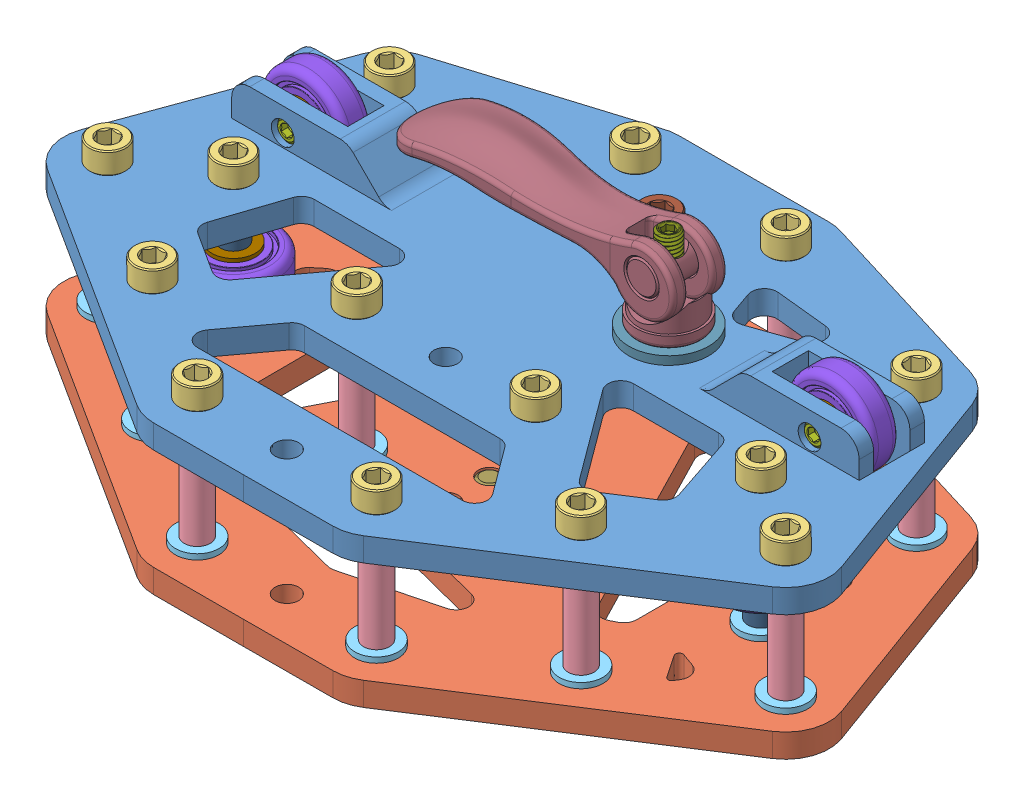
SolidWorks assembly Z-Carriage_Right, configuration Default. Lengths in mm.
Overall size (211.06 78.88 141.66).
122 component instances, 16 part files, 42 mates.
Components (placement in the parent):
- Z_Carriage_Roller_Plate_Top_B-1: Z_Carriage_Roller_Plate_Top_B [Default] at (-57.0039 2.4125 0.8021) size (210.67 16.5 141.06)
- Z_Carriage_Roller_Plate_Bottom_B-1: Z_Carriage_Roller_Plate_Bottom_B [Default] at (-56.8663 -25.5875 0.8019) x (-0.999996 0 0.002837) z (0.002837 0 0.999996) size (210.67 6.5 141.06)
- Z-Carriage_Bolt_Standoff_Assembly-1: Z-Carriage_Bolt_Standoff_Assembly [Default] at (-155.6945 -13.6491 33.5414) x (0.864384 0 -0.502833) z (0 -1 0) size (13.84 13.84 47.54)
  - 40mm_M6_Bolt-1: 40mm_M6_Bolt [96144A140] at (2.8443 6.0053 17.4384) size (10 10 46.54)
  - Z-Carriage_Standoff-1: Z-Carriage_Standoff [Default] at (2.8443 6.0053 10.4384) x (0.794662 -0.607053 0) z (0.607053 0.794662 0) size (7.14 25 7.14)
  - M6_1.5mmT_Washer-2: M6_1.5mmT_Washer [Default] at (2.8443 6.0053 -14.5616) x (1 0 0) z (0 1 0) size (12 1.5 12)
  - M6_1.5mmT_Washer-3: M6_1.5mmT_Washer [Default] at (2.8443 6.0053 11.9384) x (0.985875 0.167484 0) z (-0.167484 0.985875 0) size (12 1.5 12)
  - Nut_M6-1: Nut_M6 [91415A040] at (2.8443 6.0053 15.9384) size (10 11.55 5.56)
- Z-Carriage_Bolt_Standoff_Assembly-2: Z-Carriage_Bolt_Standoff_Assembly [Default] at (-121.3383 -13.7531 55.5414) x (0.864384 0 -0.502833) z (0 -1 0) size (13.84 13.84 47.54)
  - 40mm_M6_Bolt-1: 40mm_M6_Bolt [96144A140] at (2.8443 6.0053 17.4384) size (10 10 46.54)
  - Z-Carriage_Standoff-1: Z-Carriage_Standoff [Default] at (2.8443 6.0053 10.4384) x (0.794662 -0.607053 0) z (0.607053 0.794662 0) size (7.14 25 7.14)
  - M6_1.5mmT_Washer-2: M6_1.5mmT_Washer [Default] at (2.8443 6.0053 -14.5616) x (1 0 0) z (0 1 0) size (12 1.5 12)
  - M6_1.5mmT_Washer-3: M6_1.5mmT_Washer [Default] at (2.8443 6.0053 11.9384) x (0.985875 0.167484 0) z (-0.167484 0.985875 0) size (12 1.5 12)
  - Nut_M6-1: Nut_M6 [91415A040] at (2.8443 6.0053 15.9384) size (10 11.55 5.56)
- Z-Carriage_Bolt_Standoff_Assembly-3: Z-Carriage_Bolt_Standoff_Assembly [Default] at (-88.0491 -13.6491 80.1556) x (0.577555 0 -0.816352) z (0 -1 0) size (13.84 13.84 47.54)
  - 40mm_M6_Bolt-1: 40mm_M6_Bolt [96144A140] at (2.8443 6.0053 17.4384) size (10 10 46.54)
  - Z-Carriage_Standoff-1: Z-Carriage_Standoff [Default] at (2.8443 6.0053 10.4384) x (0.794662 -0.607053 0) z (0.607053 0.794662 0) size (7.14 25 7.14)
  - M6_1.5mmT_Washer-2: M6_1.5mmT_Washer [Default] at (2.8443 6.0053 -14.5616) x (1 0 0) z (0 1 0) size (12 1.5 12)
  - M6_1.5mmT_Washer-3: M6_1.5mmT_Washer [Default] at (2.8443 6.0053 11.9384) x (0.985875 0.167484 0) z (-0.167484 0.985875 0) size (12 1.5 12)
  - Nut_M6-1: Nut_M6 [91415A040] at (2.8443 6.0053 15.9384) size (10 11.55 5.56)
- Z-Carriage_Bolt_Standoff_Assembly-4: Z-Carriage_Bolt_Standoff_Assembly [Default] at (-37.6163 -13.6491 77.4714) x (0.864384 0 -0.502833) z (0 -1 0) size (13.84 13.84 47.54)
  - 40mm_M6_Bolt-1: 40mm_M6_Bolt [96144A140] at (2.8443 6.0053 17.4384) size (10 10 46.54)
  - Z-Carriage_Standoff-1: Z-Carriage_Standoff [Default] at (2.8443 6.0053 10.4384) x (0.794662 -0.607053 0) z (0.607053 0.794662 0) size (7.14 25 7.14)
  - M6_1.5mmT_Washer-2: M6_1.5mmT_Washer [Default] at (2.8443 6.0053 -14.5616) x (1 0 0) z (0 1 0) size (12 1.5 12)
  - M6_1.5mmT_Washer-3: M6_1.5mmT_Washer [Default] at (2.8443 6.0053 11.9384) x (0.985875 0.167484 0) z (-0.167484 0.985875 0) size (12 1.5 12)
  - Nut_M6-1: Nut_M6 [91415A040] at (2.8443 6.0053 15.9384) size (10 11.55 5.56)
- Z-Carriage_Bolt_Standoff_Assembly-5: Z-Carriage_Bolt_Standoff_Assembly [Default] at (-3.3227 -13.6491 55.374) x (0.864384 0 -0.502833) z (0 -1 0) size (13.84 13.84 47.54)
  - 40mm_M6_Bolt-1: 40mm_M6_Bolt [96144A140] at (2.8443 6.0053 17.4384) size (10 10 46.54)
  - Z-Carriage_Standoff-1: Z-Carriage_Standoff [Default] at (2.8443 6.0053 10.4384) x (0.794662 -0.607053 0) z (0.607053 0.794662 0) size (7.14 25 7.14)
  - M6_1.5mmT_Washer-2: M6_1.5mmT_Washer [Default] at (2.8443 6.0053 -14.5616) x (1 0 0) z (0 1 0) size (12 1.5 12)
  - M6_1.5mmT_Washer-3: M6_1.5mmT_Washer [Default] at (2.8443 6.0053 11.9384) x (0.985875 0.167484 0) z (-0.167484 0.985875 0) size (12 1.5 12)
  - Nut_M6-1: Nut_M6 [91415A040] at (2.8443 6.0053 15.9384) size (10 11.55 5.56)
- Z-Carriage_Bolt_Standoff_Assembly-6: Z-Carriage_Bolt_Standoff_Assembly [Default] at (30.9709 -13.6491 33.2766) x (0.864384 0 -0.502833) z (0 -1 0) size (13.84 13.84 47.54)
  - 40mm_M6_Bolt-1: 40mm_M6_Bolt [96144A140] at (2.8443 6.0053 17.4384) size (10 10 46.54)
  - Z-Carriage_Standoff-1: Z-Carriage_Standoff [Default] at (2.8443 6.0053 10.4384) x (0.794662 -0.607053 0) z (0.607053 0.794662 0) size (7.14 25 7.14)
  - M6_1.5mmT_Washer-2: M6_1.5mmT_Washer [Default] at (2.8443 6.0053 -14.5616) x (1 0 0) z (0 1 0) size (12 1.5 12)
  - M6_1.5mmT_Washer-3: M6_1.5mmT_Washer [Default] at (2.8443 6.0053 11.9384) x (0.985875 0.167484 0) z (-0.167484 0.985875 0) size (12 1.5 12)
  - Nut_M6-1: Nut_M6 [91415A040] at (2.8443 6.0053 15.9384) size (10 11.55 5.56)
- Z-Carriage_Bolt_Standoff_Assembly-7: Z-Carriage_Bolt_Standoff_Assembly [Default] at (-30.9693 -13.6491 -39.7802) x (0.206565 0 0.978433) z (0 -1 0) size (13.84 13.84 47.54)
  - 40mm_M6_Bolt-1: 40mm_M6_Bolt [96144A140] at (2.8443 6.0053 17.4384) size (10 10 46.54)
  - Z-Carriage_Standoff-1: Z-Carriage_Standoff [Default] at (2.8443 6.0053 10.4384) x (0.794662 -0.607053 0) z (0.607053 0.794662 0) size (7.14 25 7.14)
  - M6_1.5mmT_Washer-2: M6_1.5mmT_Washer [Default] at (2.8443 6.0053 -14.5616) x (1 0 0) z (0 1 0) size (12 1.5 12)
  - M6_1.5mmT_Washer-3: M6_1.5mmT_Washer [Default] at (2.8443 6.0053 11.9384) x (0.985875 0.167484 0) z (-0.167484 0.985875 0) size (12 1.5 12)
  - Nut_M6-1: Nut_M6 [91415A040] at (2.8443 6.0053 15.9384) size (10 11.55 5.56)
- Z-Carriage_Bolt_Standoff_Assembly-8: Z-Carriage_Bolt_Standoff_Assembly [Default] at (-83.1945 -13.6491 -39.4586) x (0.864384 0 -0.502833) z (0 -1 0) size (13.84 13.84 47.54)
  - 40mm_M6_Bolt-1: 40mm_M6_Bolt [96144A140] at (2.8443 6.0053 17.4384) size (10 10 46.54)
  - Z-Carriage_Standoff-1: Z-Carriage_Standoff [Default] at (2.8443 6.0053 10.4384) x (0.794662 -0.607053 0) z (0.607053 0.794662 0) size (7.14 25 7.14)
  - M6_1.5mmT_Washer-2: M6_1.5mmT_Washer [Default] at (2.8443 6.0053 -14.5616) x (1 0 0) z (0 1 0) size (12 1.5 12)
  - M6_1.5mmT_Washer-3: M6_1.5mmT_Washer [Default] at (2.8443 6.0053 11.9384) x (0.985875 0.167484 0) z (-0.167484 0.985875 0) size (12 1.5 12)
  - Nut_M6-1: Nut_M6 [91415A040] at (2.8443 6.0053 15.9384) size (10 11.55 5.56)
- Z-Carriage_Bolt_Standoff_Assembly-9: Z-Carriage_Bolt_Standoff_Assembly [Default] at (-86.9821 -13.6491 33.5414) x (0.864384 0 -0.502833) z (0 -1 0) size (13.84 13.84 47.54)
  - 40mm_M6_Bolt-1: 40mm_M6_Bolt [96144A140] at (2.8443 6.0053 17.4384) size (10 10 46.54)
  - Z-Carriage_Standoff-1: Z-Carriage_Standoff [Default] at (2.8443 6.0053 10.4384) x (0.794662 -0.607053 0) z (0.607053 0.794662 0) size (7.14 25 7.14)
  - M6_1.5mmT_Washer-2: M6_1.5mmT_Washer [Default] at (2.8443 6.0053 -14.5616) x (1 0 0) z (0 1 0) size (12 1.5 12)
  - M6_1.5mmT_Washer-3: M6_1.5mmT_Washer [Default] at (2.8443 6.0053 11.9384) x (0.985875 0.167484 0) z (-0.167484 0.985875 0) size (12 1.5 12)
  - Nut_M6-1: Nut_M6 [91415A040] at (2.8443 6.0053 15.9384) size (10 11.55 5.56)
- Z-Carriage_Bolt_Standoff_Assembly-10: Z-Carriage_Bolt_Standoff_Assembly [Default] at (-37.7411 -13.6491 33.4715) x (0.864384 0 -0.502833) z (0 -1 0) size (13.84 13.84 47.54)
  - 40mm_M6_Bolt-1: 40mm_M6_Bolt [96144A140] at (2.8443 6.0053 17.4384) size (10 10 46.54)
  - Z-Carriage_Standoff-1: Z-Carriage_Standoff [Default] at (2.8443 6.0053 10.4384) x (0.794662 -0.607053 0) z (0.607053 0.794662 0) size (7.14 25 7.14)
  - M6_1.5mmT_Washer-2: M6_1.5mmT_Washer [Default] at (2.8443 6.0053 -14.5616) x (1 0 0) z (0 1 0) size (12 1.5 12)
  - M6_1.5mmT_Washer-3: M6_1.5mmT_Washer [Default] at (2.8443 6.0053 11.9384) x (0.985875 0.167484 0) z (-0.167484 0.985875 0) size (12 1.5 12)
  - Nut_M6-1: Nut_M6 [91415A040] at (2.8443 6.0053 15.9384) size (10 11.55 5.56)
- Z-Carriage_Bolt_Standoff_Assembly-11: Z-Carriage_Bolt_Standoff_Assembly [Default] at (-135.6486 -13.6491 -17.1687) x (0.051837 0 -0.998656) z (0 -1 0) size (13.84 13.84 47.54)
  - 40mm_M6_Bolt-1: 40mm_M6_Bolt [96144A140] at (2.8443 6.0053 17.4384) size (10 10 46.54)
  - Z-Carriage_Standoff-1: Z-Carriage_Standoff [Default] at (2.8443 6.0053 10.4384) x (0.794662 -0.607053 0) z (0.607053 0.794662 0) size (7.14 25 7.14)
  - M6_1.5mmT_Washer-2: M6_1.5mmT_Washer [Default] at (2.8443 6.0053 -14.5616) x (1 0 0) z (0 1 0) size (12 1.5 12)
  - M6_1.5mmT_Washer-3: M6_1.5mmT_Washer [Default] at (2.8443 6.0053 11.9384) x (0.985875 0.167484 0) z (-0.167484 0.985875 0) size (12 1.5 12)
  - Nut_M6-1: Nut_M6 [91415A040] at (2.8443 6.0053 15.9384) size (10 11.55 5.56)
- Z-Carriage_Bolt_Standoff_Assembly-12: Z-Carriage_Bolt_Standoff_Assembly [Default] at (18.6675 -13.6491 -25.7853) x (0.600743 0 0.799443) z (0 -1 0) size (13.84 13.84 47.54)
  - 40mm_M6_Bolt-1: 40mm_M6_Bolt [96144A140] at (2.8443 6.0053 17.4384) size (10 10 46.54)
  - Z-Carriage_Standoff-1: Z-Carriage_Standoff [Default] at (2.8443 6.0053 10.4384) x (0.794662 -0.607053 0) z (0.607053 0.794662 0) size (7.14 25 7.14)
  - M6_1.5mmT_Washer-2: M6_1.5mmT_Washer [Default] at (2.8443 6.0053 -14.5616) x (1 0 0) z (0 1 0) size (12 1.5 12)
  - M6_1.5mmT_Washer-3: M6_1.5mmT_Washer [Default] at (2.8443 6.0053 11.9384) x (0.985875 0.167484 0) z (-0.167484 0.985875 0) size (12 1.5 12)
  - Nut_M6-1: Nut_M6 [91415A040] at (2.8443 6.0053 15.9384) size (10 11.55 5.56)
- Top_Bearing_Assembly-1: Top_Bearing_Assembly [Default] at (10.689 4.0604 -12.7646) size (24 24 17)
  - M6_Top_Bearing_Setscrew-1: M6_Top_Bearing_Setscrew [91390A132] at (5.1177 8.3521 14.0605) size (6.22 6.16 17)
  - Roller_Bearing_Placeholder-1: Roller_Bearing_Placeholder [Default] at (5.1177 8.3521 9.5666) x (1 0 0) z (0 -1 0) size (24 8 24)
  - M6_1mmT_Washer-1: M6_1mmT_Washer [Default] at (5.1177 8.3521 17.5666) x (-0.598252 0.801308 0) z (0.801308 0.598252 0) size (12 1 12)
  - M6_1mmT_Washer-2: M6_1mmT_Washer [Default] at (5.1177 8.3521 8.5666) x (0.928702 -0.370827 0) z (-0.370827 -0.928702 0) size (12 1 12)
- Top_Bearing_Assembly-2: Top_Bearing_Assembly [Default] at (-134.5321 4.0604 -12.7646) size (24 24 17)
  - M6_Top_Bearing_Setscrew-1: M6_Top_Bearing_Setscrew [91390A132] at (5.1177 8.3521 14.0605) size (6.22 6.16 17)
  - Roller_Bearing_Placeholder-1: Roller_Bearing_Placeholder [Default] at (5.1177 8.3521 9.5666) x (1 0 0) z (0 -1 0) size (24 8 24)
  - M6_1mmT_Washer-1: M6_1mmT_Washer [Default] at (5.1177 8.3521 17.5666) x (-0.598252 0.801308 0) z (0.801308 0.598252 0) size (12 1 12)
  - M6_1mmT_Washer-2: M6_1mmT_Washer [Default] at (5.1177 8.3521 8.5666) x (0.928702 -0.370827 0) z (-0.370827 -0.928702 0) size (12 1 12)
- Side_Bearing_Assembly-1: Side_Bearing_Assembly [Default] at (-125.5625 18.7773 -11.5921) x (0.874247 0 -0.485481) z (0.485463 -0.008727 0.874214) size (24.63 47.63 24.7)
  - 40mm_M6_Bolt-1: 40mm_M6_Bolt [96144A140] at (-20.3862 -49.6134 29.0267) x (1 0 0) z (0 -0.999962 0.008727) size (10 10 46.54)
  - M6_1.5mmT_Washer-1: M6_1.5mmT_Washer [Default] at (-20.3862 -17.6146 28.7474) x (1 0 0) z (0 0.008727 0.999962) size (12 1.5 12)
  - Roller_Bearing_Placeholder-1: Roller_Bearing_Placeholder [Default] at (-20.3862 -34.114 28.8914) x (0.999646 -0.000232 -0.026596) z (0.026597 0.008723 0.999608) size (24 8 24)
  - Z-Carriage_Standoff_Bearing-1: Z-Carriage_Standoff_Bearing [Default] at (-20.3862 -25.1143 28.8129) x (1 0 0) z (0 0.008727 0.999962) size (7.14 7.5 7.14)
  - M6_1mmT_Washer-1: M6_1mmT_Washer [Default] at (-20.3862 -26.1143 28.8216) x (0.997316 -0.000639 -0.073218) z (0.07322 0.008703 0.997278) size (12 1 12)
  - M6_1mmT_Washer-3: M6_1mmT_Washer [Default] at (-20.3862 -35.114 28.9001) x (0.947667 0.002786 0.319249) z (-0.319261 0.00827 0.947631) size (12 1 12)
  - Z-Carriage_Standoff_Bearing-3: Z-Carriage_Standoff_Bearing [Default] at (-20.3862 -42.6137 28.9656) x (1 0 0) z (0 0.008727 0.999962) size (7.14 7.5 7.14)
  - M6_1.5mmT_Washer-3: M6_1.5mmT_Washer [Default] at (-20.3862 -44.1136 28.9787) x (1 0 0) z (0 0.008727 0.999962) size (12 1.5 12)
  - Nut_M6-1: Nut_M6 [91415A040] at (-20.3862 -48.1135 29.0136) x (0.999124 -0.000365 -0.041848) z (0 -0.999962 0.008727) size (10 11.55 5.56)
- Side_Bearing_Assembly-2: Side_Bearing_Assembly [Default] at (19.6386 18.7773 -11.798) x (0.874247 0 -0.485481) z (0.485463 -0.008727 0.874214) size (24.63 47.63 24.7)
  - 40mm_M6_Bolt-1: 40mm_M6_Bolt [96144A140] at (-20.3862 -49.6134 29.0267) x (1 0 0) z (0 -0.999962 0.008727) size (10 10 46.54)
  - M6_1.5mmT_Washer-1: M6_1.5mmT_Washer [Default] at (-20.3862 -17.6146 28.7474) x (1 0 0) z (0 0.008727 0.999962) size (12 1.5 12)
  - Roller_Bearing_Placeholder-1: Roller_Bearing_Placeholder [Default] at (-20.3862 -34.114 28.8914) x (0.999646 -0.000232 -0.026596) z (0.026597 0.008723 0.999608) size (24 8 24)
  - Z-Carriage_Standoff_Bearing-1: Z-Carriage_Standoff_Bearing [Default] at (-20.3862 -25.1143 28.8129) x (1 0 0) z (0 0.008727 0.999962) size (7.14 7.5 7.14)
  - M6_1mmT_Washer-1: M6_1mmT_Washer [Default] at (-20.3862 -26.1143 28.8216) x (0.997316 -0.000639 -0.073218) z (0.07322 0.008703 0.997278) size (12 1 12)
  - M6_1mmT_Washer-3: M6_1mmT_Washer [Default] at (-20.3862 -35.114 28.9001) x (0.947667 0.002786 0.319249) z (-0.319261 0.00827 0.947631) size (12 1 12)
  - Z-Carriage_Standoff_Bearing-3: Z-Carriage_Standoff_Bearing [Default] at (-20.3862 -42.6137 28.9656) x (1 0 0) z (0 0.008727 0.999962) size (7.14 7.5 7.14)
  - M6_1.5mmT_Washer-3: M6_1.5mmT_Washer [Default] at (-20.3862 -44.1136 28.9787) x (1 0 0) z (0 0.008727 0.999962) size (12 1.5 12)
  - Nut_M6-1: Nut_M6 [91415A040] at (-20.3862 -48.1135 29.0136) x (0.999124 -0.000365 -0.041848) z (0 -0.999962 0.008727) size (10 11.55 5.56)
- Idler_Bearing_Assembly-1: Idler_Bearing_Assembly [Default] at (-86.4176 18.7773 -2.3736) x (-0.930317 0 -0.366758) z (0.366744 -0.008727 -0.930281) size (24.63 56.64 24.7)
  - M6_1.5mmT_Washer-1: M6_1.5mmT_Washer [Default] at (-20.3135 -17.6139 28.8293) x (1 0 0) z (0 0.008727 0.999962) size (12 1.5 12)
  - Roller_Bearing_Placeholder-1: Roller_Bearing_Placeholder [Default] at (-20.3135 -34.1133 28.9733) x (0.999646 -0.000232 -0.026596) z (0.026597 0.008723 0.999608) size (24 8 24)
  - Z-Carriage_Standoff_Bearing-1: Z-Carriage_Standoff_Bearing [Default] at (-20.3135 -25.1136 28.8947) x (1 0 0) z (0 0.008727 0.999962) size (7.14 7.5 7.14)
  - M6_1mmT_Washer-1: M6_1mmT_Washer [Default] at (-20.3135 -26.1136 28.9035) x (0.997316 -0.000639 -0.073218) z (0.07322 0.008703 0.997278) size (12 1 12)
  - M6_1mmT_Washer-3: M6_1mmT_Washer [Default] at (-20.3135 -35.1132 28.982) x (0.947667 0.002786 0.319249) z (-0.319261 0.00827 0.947631) size (12 1 12)
  - Z-Carriage_Standoff_Bearing-3: Z-Carriage_Standoff_Bearing [Default] at (-20.3862 -42.6137 28.9656) x (1 0 0) z (0 0.008727 0.999962) size (7.14 7.5 7.14)
  - M6_1.5mmT_Washer-3: M6_1.5mmT_Washer [Default] at (-20.3135 -44.1129 29.0605) x (1 0 0) z (0 0.008727 0.999962) size (12 1.5 12)
  - M6_1.5mmT_Washer-4: M6_1.5mmT_Washer [Default] at (-20.3135 -52.1126 29.1303) x (1 0 0) z (0 0.008727 0.999962) size (12 1.5 12)
  - 50mm_M6_Bolt-1: 50mm_M6_Bolt [96144A150] at (-20.3135 -59.6123 29.1958) x (0.957975 0.002503 0.286842) z (0 -0.999962 0.008727) size (10 10 56.54)
  - Nut_M6-2: Nut_M6 [91415A040] at (-20.3135 -57.1124 29.174) x (0.997327 0.000638 0.073062) z (0 -0.999962 0.008727) size (10 11.55 5.56)
- Nut_M6-1: Nut_M6 [91415A040] at (-56.9003 -29.5875 25.3021) x (1 0 0) z (0 -1 0) size (10 11.55 5.56)
- 12mm_M6_Bolt-1: 12mm_M6_Bolt [96144A111] at (-56.9003 -25.5875 25.3021) x (1 0 0) z (0 1 0) size (10 10 18.46)
- Cam_Lock_Assembly-1: Cam_Lock_Assembly [Default] at (-91.2895 -17.7473 -62.7012) size (96.09 41 24.66)
  - Cam_Lock-1: Cam_Lock [2030N21] at (59.2856 28.9599 63.5033) size (80.06 22.06 23.66)
  - M6_Fender_Washer-1: M6_Fender_Washer [98363A112] at (59.2856 26.6599 63.5033) x (0.991616 0 -0.129221) z (0 1 0) size (22 22 2.3)
  - Cam_Lock_Nut-1: Cam_Lock_Nut [Default] at (84.2833 7.0599 63.8438) x (-0.01362 0 0.999907) z (-0.999907 0 -0.01362) size (11.58 4.64 50)
  - 40mm_M6x1_Cam_Lock_Bolt-1: 40mm_M6x1_Cam_Lock_Bolt [92015A558] at (59.2856 32.2406 63.5033) x (0.997508 0 -0.070558) z (0 1 0) size (6.22 6.16 41)
Mates (geometry in assembly coordinates):
- Distance1: distance = 28 mm anti-aligned: plane of Z_Carriage_Roller_Plate_Bottom_B-1 through (-150.2162 -25.5875 37.3021) normal (0 1 0); plane of Z_Carriage_Roller_Plate_Top_B-1 through (36.4492 2.4125 37.0373) normal (0 -1 0)
- Concentric3: concentric aligned: circle of Z_Carriage_Roller_Plate_Top_B-1; circle of Z-Carriage_Bolt_Standoff_Assembly-1/M6_1.5mmT_Washer-2
- Coincident1: coincident anti-aligned: plane of Z_Carriage_Roller_Plate_Top_B-1 through (36.4492 2.4125 37.0373) normal (0 -1 0); plane of Z-Carriage_Bolt_Standoff_Assembly-1/M6_1.5mmT_Washer-2 through (-150.2162 2.4125 37.3021) normal (0 1 0)
- Concentric4: concentric anti-aligned: circle of Z_Carriage_Roller_Plate_Top_B-1; circle of Z_Carriage_Roller_Plate_Bottom_B-1
- Concentric5: concentric anti-aligned: circle of Z_Carriage_Roller_Plate_Top_B-1; circle of Z_Carriage_Roller_Plate_Bottom_B-1
- Concentric6: concentric aligned: circle of Z_Carriage_Roller_Plate_Top_B-1; circle of Z-Carriage_Bolt_Standoff_Assembly-2/M6_1.5mmT_Washer-2
- Concentric7: concentric aligned: circle of Z_Carriage_Roller_Plate_Top_B-1; circle of Z-Carriage_Bolt_Standoff_Assembly-3/M6_1.5mmT_Washer-2
- Concentric8: concentric aligned: circle of Z_Carriage_Roller_Plate_Top_B-1; circle of Z-Carriage_Bolt_Standoff_Assembly-4/M6_1.5mmT_Washer-2
- Concentric9: concentric aligned: circle of Z_Carriage_Roller_Plate_Top_B-1; circle of Z-Carriage_Bolt_Standoff_Assembly-5/M6_1.5mmT_Washer-2
- Concentric10: concentric aligned: circle of Z_Carriage_Roller_Plate_Top_B-1; circle of Z-Carriage_Bolt_Standoff_Assembly-6/M6_1.5mmT_Washer-2
- Concentric11: concentric aligned: circle of Z_Carriage_Roller_Plate_Top_B-1; circle of Z-Carriage_Bolt_Standoff_Assembly-7/M6_1.5mmT_Washer-2
- Concentric12: concentric aligned: circle of Z_Carriage_Roller_Plate_Top_B-1; circle of Z-Carriage_Bolt_Standoff_Assembly-8/M6_1.5mmT_Washer-2
- Concentric13: concentric aligned: circle of Z_Carriage_Roller_Plate_Top_B-1; circle of Z-Carriage_Bolt_Standoff_Assembly-9/40mm_M6_Bolt-1
- Concentric14: concentric aligned: circle of Z_Carriage_Roller_Plate_Top_B-1; circle of Z-Carriage_Bolt_Standoff_Assembly-10/M6_1.5mmT_Washer-2
- Coincident2: coincident aligned: plane of Z-Carriage_Bolt_Standoff_Assembly-3/M6_1.5mmT_Washer-2 through (-81.5039 2.4125 81.3021) normal (0 1 0); plane of Z-Carriage_Bolt_Standoff_Assembly-4/M6_1.5mmT_Washer-2 through (-32.138 2.4125 81.232) normal (0 1 0)
- Coincident3: coincident aligned: plane of Z-Carriage_Bolt_Standoff_Assembly-3/M6_1.5mmT_Washer-2 through (-81.5039 2.4125 81.3021) normal (0 1 0); plane of Z-Carriage_Bolt_Standoff_Assembly-5/M6_1.5mmT_Washer-2 through (2.1556 2.4125 59.1347) normal (0 1 0)
- Coincident4: coincident aligned: plane of Z-Carriage_Bolt_Standoff_Assembly-3/M6_1.5mmT_Washer-2 through (-81.5039 2.4125 81.3021) normal (0 1 0); plane of Z-Carriage_Bolt_Standoff_Assembly-6/M6_1.5mmT_Washer-2 through (36.4492 2.4125 37.0373) normal (0 1 0)
- Coincident5: coincident aligned: plane of Z-Carriage_Bolt_Standoff_Assembly-3/M6_1.5mmT_Washer-2 through (-81.5039 2.4125 81.3021) normal (0 1 0); plane of Z-Carriage_Bolt_Standoff_Assembly-10/M6_1.5mmT_Washer-2 through (-32.2628 2.4125 37.2322) normal (0 1 0)
- Coincident6: coincident aligned: plane of Z-Carriage_Bolt_Standoff_Assembly-3/M6_1.5mmT_Washer-2 through (-81.5039 2.4125 81.3021) normal (0 1 0); plane of Z-Carriage_Bolt_Standoff_Assembly-9/M6_1.5mmT_Washer-2 through (-81.5039 2.4125 37.3021) normal (0 1 0)
- Coincident7: coincident aligned: plane of Z-Carriage_Bolt_Standoff_Assembly-3/M6_1.5mmT_Washer-2 through (-81.5039 2.4125 81.3021) normal (0 1 0); plane of Z-Carriage_Bolt_Standoff_Assembly-8/M6_1.5mmT_Washer-2 through (-77.7162 2.4125 -35.6979) normal (0 1 0)
- Coincident8: coincident aligned: plane of Z-Carriage_Bolt_Standoff_Assembly-3/M6_1.5mmT_Washer-2 through (-81.5039 2.4125 81.3021) normal (0 1 0); plane of Z-Carriage_Bolt_Standoff_Assembly-7/M6_1.5mmT_Washer-2 through (-36.2576 2.4125 -35.7567) normal (0 1 0)
- Coincident10: coincident anti-aligned: plane of Z_Carriage_Roller_Plate_Top_B-1 through (36.4492 2.4125 37.0373) normal (0 -1 0); plane of Z-Carriage_Bolt_Standoff_Assembly-3/M6_1.5mmT_Washer-2 through (-81.5039 2.4125 81.3021) normal (0 1 0)
- Concentric15: concentric aligned: circle of Z_Carriage_Roller_Plate_Top_B-1; circle of Z-Carriage_Bolt_Standoff_Assembly-11/M6_1.5mmT_Washer-2
- Concentric16: concentric aligned: circle of Z_Carriage_Roller_Plate_Top_B-1; circle of Z-Carriage_Bolt_Standoff_Assembly-12/M6_1.5mmT_Washer-2
- Coincident11: coincident anti-aligned: plane of Z_Carriage_Roller_Plate_Top_B-1 through (36.4492 2.4125 37.0373) normal (0 -1 0); plane of Z-Carriage_Bolt_Standoff_Assembly-12/M6_1.5mmT_Washer-2 through (15.5753 2.4125 -19.9037) normal (0 1 0)
- Coincident12: coincident anti-aligned: plane of Z_Carriage_Roller_Plate_Top_B-1 through (36.4492 2.4125 37.0373) normal (0 -1 0); plane of Z-Carriage_Bolt_Standoff_Assembly-11/M6_1.5mmT_Washer-2 through (-129.5039 2.4125 -19.6979) normal (0 1 0)
- Concentric21: concentric aligned: circle of Z_Carriage_Roller_Plate_Top_B-1; circle of Top_Bearing_Assembly-1/M6_1mmT_Washer-1
- Distance5: distance = 1 mm aligned: plane of Top_Bearing_Assembly-1/M6_Top_Bearing_Setscrew-1 through (15.8067 12.4125 8.8021) normal (0 0 1); plane of Z_Carriage_Roller_Plate_Top_B-1 through (29.4961 18.9125 9.8021) normal (0 0 1)
- Concentric22: concentric aligned: circle of Z_Carriage_Roller_Plate_Top_B-1; circle of Top_Bearing_Assembly-2/M6_1mmT_Washer-1
- Distance6: distance = 1 mm aligned: plane of Top_Bearing_Assembly-2/M6_Top_Bearing_Setscrew-1 through (-129.4144 12.4125 8.8021) normal (0 0 1); plane of Z_Carriage_Roller_Plate_Top_B-1 through (-115.5039 18.9125 9.8021) normal (0 0 1)
- Coincident16: coincident anti-aligned: plane of Z_Carriage_Roller_Plate_Top_B-1 through (36.4492 2.4125 37.0373) normal (0 -1 0); plane of Side_Bearing_Assembly-1/M6_1.5mmT_Washer-1 through (-129.5039 2.4125 23.3021) normal (0 1 0)
- Concentric23: concentric anti-aligned: cylinder of Z_Carriage_Roller_Plate_Top_B-1 through (-129.5039 8.9125 23.3021) axis (0 -1 0) radius 3.15; circle of Side_Bearing_Assembly-1/M6_1.5mmT_Washer-1
- Coincident17: coincident anti-aligned: plane of Z_Carriage_Roller_Plate_Top_B-1 through (36.4492 2.4125 37.0373) normal (0 -1 0); plane of Side_Bearing_Assembly-2/M6_1.5mmT_Washer-1 through (15.6973 2.4125 23.0961) normal (0 1 0)
- Concentric24: concentric aligned: circle of Z_Carriage_Roller_Plate_Top_B-1; circle of Side_Bearing_Assembly-2/M6_1.5mmT_Washer-1
- Coincident18: coincident anti-aligned: plane of Z_Carriage_Roller_Plate_Top_B-1 through (36.4492 2.4125 37.0373) normal (0 -1 0); plane of Idler_Bearing_Assembly-1/M6_1.5mmT_Washer-1 through (-57.003 2.4125 -21.5998) normal (0 1 0)
- Slot1: slot aligned: cylinder of Idler_Bearing_Assembly-1/50mm_M6_Bolt-1 through (-57.003 8.9125 -21.5998) axis (0 -1 0) radius 3; cylinder of Z_Carriage_Roller_Plate_Top_B-1 through (-57.0478 8.9125 -26.6979) axis (0 -1 0) radius 3.15; cylinder of Z_Carriage_Roller_Plate_Top_B-1 through (-56.9599 8.9125 -16.6979) axis (0 -1 0) radius 3.15
- Coincident19: coincident aligned: plane of Z_Carriage_Roller_Plate_Bottom_B-1 through (-150.2162 -32.0875 37.3021) normal (0 -1 0); plane of Nut_M6-1 through (-61.9003 -32.0875 28.1888) normal (0 -1 0)
- Concentric25: concentric anti-aligned: cylinder of Z_Carriage_Roller_Plate_Bottom_B-1 through (-56.9003 -32.0875 25.3021) axis (0 1 0) radius 3.1; circle of Nut_M6-1
- Coincident20: coincident aligned: plane of Z_Carriage_Roller_Plate_Bottom_B-1 through (-150.2162 -25.5875 37.3021) normal (0 1 0); circle of 12mm_M6_Bolt-1
- Concentric26: concentric anti-aligned: circle of Nut_M6-1; circle of 12mm_M6_Bolt-1
- Concentric27: concentric aligned: circle of Z_Carriage_Roller_Plate_Top_B-1; circle of Cam_Lock_Assembly-1/M6_Fender_Washer-1
- Coincident21: coincident anti-aligned: plane of Z_Carriage_Roller_Plate_Top_B-1 through (36.4492 8.9125 37.0373) normal (0 1 0); plane of Cam_Lock_Assembly-1/M6_Fender_Washer-1 through (-32.0039 8.9125 0.8021) normal (0 -1 0)
